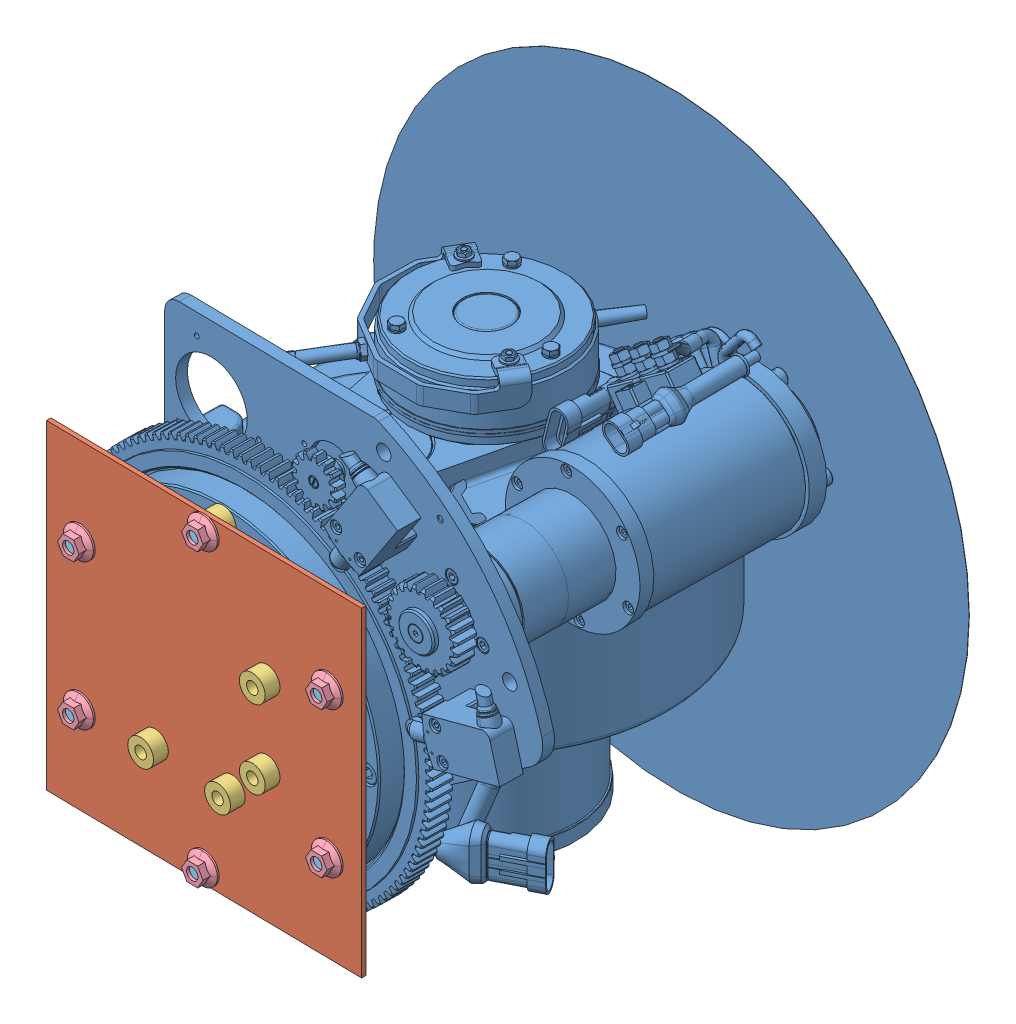
SolidWorks assembly motore+supporto, configuration Default. Lengths in mm.
Overall size (415.84 415.9 330.44).
29 component instances, 5 part files, 56 mates.
Components (placement in the parent):
- MR240FRS-AC.stp-1: MR240FRS-AC.stp [Default] at (480.9296 100.5307 -916.9118) size (415.84 415.9 312.91)
- supporto_motore-2: supporto_motore [Default] at (5.5916 0.2825 575.9688) x (-0.999869 0 -0.016207) z (0.016207 -0.000006 -0.999869) size (220 220 3)
- distanziale-1: distanziale [Default] at (92.3448 50.2824 567.3735) x (0.92025 -0.391047 0.014919) z (-0.016207 0.000006 0.999869) size (18 18 10)
- distanziale-2: distanziale [Default] at (-80.8375 -49.7176 564.5668) x (-0.654362 0.756107 -0.010611) z (-0.016207 0.000006 0.999869) size (18 18 10)
- distanziale-3: distanziale [Default] at (5.7536 -99.7176 565.9707) x (-0.654362 0.756107 -0.010611) z (-0.016207 0.000006 0.999869) size (18 18 10)
- distanziale-4: distanziale [Default] at (5.5916 100.2825 575.9683) x (-0.701568 -0.712512 -0.011368) z (0.016207 -0.000006 -0.999869) size (18 18 10)
- distanziale-5: distanziale [Default] at (92.3448 -49.7176 567.374) x (-0.654362 0.756107 -0.010611) z (-0.016207 0.000006 0.999869) size (18 18 10)
- distanziale-6: distanziale [Default] at (-80.8375 50.2824 564.5663) x (0.92025 -0.391047 0.014919) z (-0.016207 0.000006 0.999869) size (18 18 10)
- distanziale-7: distanziale [Default] at (-28.6146 -43.7175 588.4163) x (0.316566 0.948557 0.005126) z (0.016207 -0.000006 -0.999869) size (18 18 10)
- distanziale-8: distanziale [Default] at (49.3751 34.2825 589.6801) x (0.316566 0.948557 0.005126) z (0.016207 -0.000006 -0.999869) size (18 18 10)
- distanziale-9: distanziale [Default] at (25.1283 -43.7175 589.2875) x (-0.701568 -0.712512 -0.011368) z (0.016207 -0.000006 -0.999869) size (18 18 10)
- FLANGE_NUT_M8-1: FLANGE_NUT_M8 [Default] at (92.1341 -49.7175 580.3723) x (0.999869 0 0.016207) z (-0.016207 0.000006 0.999869) size (21 21 8)
- FLANGE_NUT_M8-2: FLANGE_NUT_M8 [Default] at (-81.0482 50.2825 577.5646) x (0.999869 0 0.016207) z (-0.016207 0.000006 0.999869) size (21 21 8)
- FLANGE_NUT_M8-3: FLANGE_NUT_M8 [Default] at (-81.0482 -49.7175 577.5651) x (0.999869 0 0.016207) z (-0.016207 0.000006 0.999869) size (21 21 8)
- FLANGE_NUT_M8-4: FLANGE_NUT_M8 [Default] at (5.5429 -99.7175 578.969) x (0.999869 0 0.016207) z (-0.016207 0.000006 0.999869) size (21 21 8)
- FLANGE_NUT_M8-5: FLANGE_NUT_M8 [Default] at (5.543 100.2825 578.9679) x (0.999869 0 0.016207) z (-0.016207 0.000006 0.999869) size (21 21 8)
- FLANGE_NUT_M8-6: FLANGE_NUT_M8 [Default] at (92.1342 50.2825 580.3717) x (0.999869 0 0.016207) z (-0.016207 0.000006 0.999869) size (21 21 8)
- FLANGE_NUT_M8-7: FLANGE_NUT_M8 [Default] at (-28.4039 -43.7175 575.418) x (-0.924292 -0.381392 -0.01498) z (0.016207 -0.000006 -0.999869) size (21 21 8)
- FLANGE_NUT_M8-8: FLANGE_NUT_M8 [Default] at (25.339 -43.7175 576.2892) x (0.999868 -0.000687 0.016207) z (0.016207 -0.000006 -0.999869) size (21 21 8)
- FLANGE_NUT_M8-9: FLANGE_NUT_M8 [Default] at (49.5858 34.2825 576.6818) x (-0.924292 -0.381392 -0.01498) z (0.016207 -0.000006 -0.999869) size (21 21 8)
- slotted countersunk flat head screw_iso-1: slotted countersunk flat head screw_iso [ISO 2009 - M8 x 50 - 38N] at (-80.3351 -49.7178 533.5709) x (-0.016207 0.000006 0.999869) z (-0.999869 -0.000006 -0.016207) size (50 15.8 15.67)
- slotted countersunk flat head screw_iso-2: slotted countersunk flat head screw_iso [ISO 2009 - M8 x 50 - 38N] at (-3.804 -13.9391 527.2162) size (50 15.8 15.67)
- slotted countersunk flat head screw_iso-4: slotted countersunk flat head screw_iso [ISO 2009 - M8 x 50 - 38N] at (6.2561 -99.7178 534.9748) x (-0.016207 0.000006 0.999869) z (-0.999869 -0.000006 -0.016207) size (50 15.8 15.67)
- slotted countersunk flat head screw_iso-5: slotted countersunk flat head screw_iso [ISO 2009 - M8 x 50 - 38N] at (92.8472 -49.7178 536.3781) x (-0.016207 0.000006 0.999869) z (-0.999869 -0.000006 -0.016207) size (50 15.8 15.67)
- slotted countersunk flat head screw_iso-6: slotted countersunk flat head screw_iso [ISO 2009 - M8 x 50 - 38N] at (-80.3351 50.2822 533.5704) x (-0.016207 0.000006 0.999869) z (-0.999869 -0.000006 -0.016207) size (50 15.8 15.67)
- slotted countersunk flat head screw_iso-7: slotted countersunk flat head screw_iso [ISO 2009 - M8 x 50 - 38N] at (6.2561 100.2822 534.9737) x (-0.016207 0.000006 0.999869) z (-0.999869 -0.000006 -0.016207) size (50 15.8 15.67)
- slotted countersunk flat head screw_iso-8: slotted countersunk flat head screw_iso [ISO 2009 - M8 x 50 - 38N] at (92.8473 50.2822 536.3775) x (-0.016207 0.000006 0.999869) z (-0.999869 -0.000006 -0.016207) size (50 15.8 15.67)
- distanziale-10: distanziale [Default] at (49.3751 -19.4675 589.6804) x (-0.807591 -0.589598 -0.013087) z (0.016207 -0.000006 -0.999869) size (18 18 10)
- FLANGE_NUT_M8-10: FLANGE_NUT_M8 [Default] at (49.5858 -19.4675 576.6821) x (-0.924292 -0.381392 -0.01498) z (0.016207 -0.000006 -0.999869) size (21 21 8)
Mates (geometry in assembly coordinates):
- Concentrico1: concentric aligned: cylinder of supporto_motore-2 through (92.1342 50.2825 580.3717) axis (0.016207 -0.000006 -0.999869) radius 4; cylinder of distanziale-1 through (92.1828 50.2824 577.3721) axis (0.016207 -0.000006 -0.999869) radius 4
- Coincidente1: coincident anti-aligned: plane of supporto_motore-2 through (5.5916 0.2825 575.9688) normal (0.016207 -0.000006 -0.999869); plane of distanziale-1 through (92.1828 50.2824 577.3721) normal (-0.016207 0.000006 0.999869)
- Coincidente2: coincident anti-aligned: plane of supporto_motore-2 through (5.5916 0.2825 575.9688) normal (0.016207 -0.000006 -0.999869); plane of distanziale-4 through (5.5916 100.2825 575.9683) normal (-0.016207 0.000006 0.999869)
- Concentrico2: concentric anti-aligned: cylinder of supporto_motore-2 through (5.543 100.2825 578.9679) axis (0.016207 -0.000006 -0.999869) radius 4; cylinder of distanziale-4 through (5.7537 100.2824 565.9696) axis (-0.016207 0.000006 0.999869) radius 4
- Coincidente3: coincident anti-aligned: plane of supporto_motore-2 through (5.5916 0.2825 575.9688) normal (0.016207 -0.000006 -0.999869); plane of distanziale-6 through (-80.9996 50.2825 574.565) normal (-0.016207 0.000006 0.999869)
- Concentrico3: concentric aligned: cylinder of supporto_motore-2 through (-81.0482 50.2825 577.5646) axis (0.016207 -0.000006 -0.999869) radius 4; cylinder of distanziale-6 through (-80.9996 50.2825 574.565) axis (0.016207 -0.000006 -0.999869) radius 4
- Concentrico4: concentric aligned: cylinder of supporto_motore-2 through (-81.0482 -49.7175 577.5651) axis (0.016207 -0.000006 -0.999869) radius 4; cylinder of distanziale-2 through (-80.9996 -49.7175 574.5655) axis (0.016207 -0.000006 -0.999869) radius 4
- Coincidente4: coincident anti-aligned: plane of supporto_motore-2 through (5.5916 0.2825 575.9688) normal (0.016207 -0.000006 -0.999869); plane of distanziale-2 through (-80.9996 -49.7175 574.5655) normal (-0.016207 0.000006 0.999869)
- Coincidente5: coincident anti-aligned: plane of supporto_motore-2 through (5.5916 0.2825 575.9688) normal (0.016207 -0.000006 -0.999869); plane of distanziale-3 through (5.5916 -99.7175 575.9694) normal (-0.016207 0.000006 0.999869)
- Concentrico5: concentric aligned: cylinder of supporto_motore-2 through (5.5429 -99.7175 578.969) axis (0.016207 -0.000006 -0.999869) radius 4; cylinder of distanziale-3 through (5.5916 -99.7175 575.9694) axis (0.016207 -0.000006 -0.999869) radius 4
- Coincidente6: coincident anti-aligned: plane of supporto_motore-2 through (5.5916 0.2825 575.9688) normal (0.016207 -0.000006 -0.999869); plane of distanziale-5 through (92.1827 -49.7176 577.3727) normal (-0.016207 0.000006 0.999869)
- Concentrico6: concentric aligned: cylinder of supporto_motore-2 through (92.1341 -49.7175 580.3723) axis (0.016207 -0.000006 -0.999869) radius 4; cylinder of distanziale-5 through (92.1827 -49.7176 577.3727) axis (0.016207 -0.000006 -0.999869) radius 4
- Concentrico7: concentric anti-aligned: cylinder of MR240FRS-AC.stp-1 through (10.7642 -99.7193 256.856) axis (-0.016207 0.000006 0.999869) radius 3.3235; cylinder of distanziale-3 through (5.5916 -99.7175 575.9694) axis (0.016207 -0.000006 -0.999869) radius 4
- Concentrico8: concentric aligned: cylinder of MR240FRS-AC.stp-1 through (10.7642 100.2807 256.8549) axis (-0.016207 0.000006 0.999869) radius 3.3235; cylinder of distanziale-4 through (5.7537 100.2824 565.9696) axis (-0.016207 0.000006 0.999869) radius 4
- Coincidente7: coincident anti-aligned: plane of MR240FRS-AC.stp-1 through (102.7409 0.2824 567.5422) normal (-0.016207 0.000006 0.999869); plane of distanziale-3 through (5.7536 -99.7176 565.9707) normal (0.016207 -0.000006 -0.999869)
- Coincidente9: coincident anti-aligned: plane of supporto_motore-2 through (5.543 0.2825 578.9684) normal (-0.016207 0.000006 0.999869); plane of distanziale-8 through (49.5372 34.2825 579.6814) normal (0.016207 -0.000006 -0.999869)
- Coincidente10: coincident anti-aligned: plane of supporto_motore-2 through (5.543 0.2825 578.9684) normal (-0.016207 0.000006 0.999869); plane of distanziale-7 through (-28.4526 -43.7175 578.4176) normal (0.016207 -0.000006 -0.999869)
- Coincidente11: coincident anti-aligned: plane of supporto_motore-2 through (5.543 0.2825 578.9684) normal (-0.016207 0.000006 0.999869); plane of distanziale-9 through (25.2904 -43.7175 579.2888) normal (0.016207 -0.000006 -0.999869)
- Concentrico10: concentric anti-aligned: cylinder of supporto_motore-2 through (-28.4526 -43.7175 578.4176) axis (0.016207 -0.000006 -0.999869) radius 4; cylinder of distanziale-7 through (-28.4526 -43.7175 578.4176) axis (-0.016207 0.000006 0.999869) radius 4
- Concentrico11: concentric anti-aligned: cylinder of supporto_motore-2 through (25.2904 -43.7175 579.2888) axis (0.016207 -0.000006 -0.999869) radius 4; cylinder of distanziale-9 through (25.2904 -43.7175 579.2888) axis (-0.016207 0.000006 0.999869) radius 4
- Concentrico12: concentric anti-aligned: cylinder of supporto_motore-2 through (49.5372 34.2825 579.6814) axis (0.016207 -0.000006 -0.999869) radius 4; cylinder of distanziale-8 through (49.5372 34.2825 579.6814) axis (-0.016207 0.000006 0.999869) radius 4
- Concentrico13: concentric aligned: cylinder of supporto_motore-2 through (25.2904 -43.7175 579.2888) axis (0.016207 -0.000006 -0.999869) radius 4; cylinder of FLANGE_NUT_M8-8 through (25.4751 -43.7176 567.8903) axis (0.016207 -0.000006 -0.999869) radius 4
- Coincidente12: coincident anti-aligned: plane of supporto_motore-2 through (5.5916 0.2825 575.9688) normal (0.016207 -0.000006 -0.999869); plane of FLANGE_NUT_M8-8 through (36.8954 -32.1755 576.4764) normal (-0.016207 0.000006 0.999869)
- Coincidente13: coincident anti-aligned: plane of supporto_motore-2 through (5.5916 0.2825 575.9688) normal (0.016207 -0.000006 -0.999869); plane of FLANGE_NUT_M8-9 through (43.3148 19.2004 576.5802) normal (-0.016207 0.000006 0.999869)
- Concentrico14: concentric aligned: cylinder of supporto_motore-2 through (49.5372 34.2825 579.6814) axis (0.016207 -0.000006 -0.999869) radius 4; cylinder of FLANGE_NUT_M8-9 through (49.722 34.2824 568.2829) axis (0.016207 -0.000006 -0.999869) radius 4
- Coincidente14: coincident anti-aligned: plane of supporto_motore-2 through (5.5916 0.2825 575.9688) normal (0.016207 -0.000006 -0.999869); plane of FLANGE_NUT_M8-7 through (-34.675 -58.7996 575.3165) normal (-0.016207 0.000006 0.999869)
- Concentrico15: concentric aligned: cylinder of supporto_motore-2 through (-28.4526 -43.7175 578.4176) axis (0.016207 -0.000006 -0.999869) radius 4; cylinder of FLANGE_NUT_M8-7 through (-28.2678 -43.7176 567.0191) axis (0.016207 -0.000006 -0.999869) radius 4
- Coincidente15: coincident anti-aligned: plane of supporto_motore-2 through (5.543 0.2825 578.9684) normal (-0.016207 0.000006 0.999869); plane of FLANGE_NUT_M8-4 through (17.0914 -111.2675 579.1563) normal (0.016207 -0.000006 -0.999869)
- Coincidente16: coincident anti-aligned: plane of supporto_motore-2 through (5.543 0.2825 578.9684) normal (-0.016207 0.000006 0.999869); plane of FLANGE_NUT_M8-1 through (103.6826 -61.2675 580.5596) normal (0.016207 -0.000006 -0.999869)
- Coincidente17: coincident anti-aligned: plane of supporto_motore-2 through (5.543 0.2825 578.9684) normal (-0.016207 0.000006 0.999869); plane of FLANGE_NUT_M8-5 through (17.0915 88.7325 579.1551) normal (0.016207 -0.000006 -0.999869)
- Coincidente18: coincident anti-aligned: plane of supporto_motore-2 through (5.543 0.2825 578.9684) normal (-0.016207 0.000006 0.999869); plane of FLANGE_NUT_M8-6 through (103.6826 38.7325 580.559) normal (0.016207 -0.000006 -0.999869)
- Coincidente19: coincident anti-aligned: plane of supporto_motore-2 through (5.543 0.2825 578.9684) normal (-0.016207 0.000006 0.999869); plane of FLANGE_NUT_M8-3 through (-69.4997 -61.2675 577.7524) normal (0.016207 -0.000006 -0.999869)
- Coincidente20: coincident anti-aligned: plane of supporto_motore-2 through (5.543 0.2825 578.9684) normal (-0.016207 0.000006 0.999869); plane of FLANGE_NUT_M8-2 through (-69.4997 38.7325 577.7518) normal (0.016207 -0.000006 -0.999869)
- Concentrico16: concentric anti-aligned: cylinder of supporto_motore-2 through (-81.0482 -49.7175 577.5651) axis (0.016207 -0.000006 -0.999869) radius 4; cylinder of FLANGE_NUT_M8-3 through (-81.1843 -49.7175 585.964) axis (-0.016207 0.000006 0.999869) radius 4
- Concentrico17: concentric anti-aligned: cylinder of supporto_motore-2 through (-81.0482 50.2825 577.5646) axis (0.016207 -0.000006 -0.999869) radius 4; cylinder of FLANGE_NUT_M8-2 through (-81.1843 50.2825 585.9635) axis (-0.016207 0.000006 0.999869) radius 4
- Concentrico18: concentric anti-aligned: cylinder of supporto_motore-2 through (5.543 100.2825 578.9679) axis (0.016207 -0.000006 -0.999869) radius 4; cylinder of FLANGE_NUT_M8-5 through (5.4069 100.2825 587.3668) axis (-0.016207 0.000006 0.999869) radius 4
- Concentrico19: concentric anti-aligned: cylinder of supporto_motore-2 through (92.1342 50.2825 580.3717) axis (0.016207 -0.000006 -0.999869) radius 4; cylinder of FLANGE_NUT_M8-6 through (91.998 50.2825 588.7706) axis (-0.016207 0.000006 0.999869) radius 4
- Concentrico20: concentric anti-aligned: cylinder of supporto_motore-2 through (92.1341 -49.7175 580.3723) axis (0.016207 -0.000006 -0.999869) radius 4; cylinder of FLANGE_NUT_M8-1 through (91.998 -49.7175 588.7712) axis (-0.016207 0.000006 0.999869) radius 4
- Concentrico21: concentric anti-aligned: cylinder of supporto_motore-2 through (5.5429 -99.7175 578.969) axis (0.016207 -0.000006 -0.999869) radius 4; cylinder of FLANGE_NUT_M8-4 through (5.4068 -99.7175 587.3679) axis (-0.016207 0.000006 0.999869) radius 4
- Concentrico22: concentric aligned: cylinder of MR240FRS-AC.stp-1 through (-74.6264 -49.7197 181.3862) axis (-0.016207 0.000006 0.999869) radius 4.5; cone of slotted countersunk flat head screw_iso-1 through (-80.3472 -49.7177 534.3208) axis (-0.016207 0.000006 0.999869)
- Coincidente21: coincident aligned: plane of MR240FRS-AC.stp-1 through (-94.2307 0.2823 533.3454) normal (0.016207 -0.000006 -0.999869); plane of slotted countersunk flat head screw_iso-1 through (-80.3351 -49.7178 533.5709) normal (0.016207 -0.000006 -0.999869)
- Concentrico23: concentric aligned: cylinder of MR240FRS-AC.stp-1 through (11.9647 -99.7197 182.7901) axis (-0.016207 0.000006 0.999869) radius 4.5; cone of slotted countersunk flat head screw_iso-4 through (6.2439 -99.7178 535.7247) axis (-0.016207 0.000006 0.999869)
- Concentrico24: concentric aligned: cylinder of MR240FRS-AC.stp-1 through (98.5559 -49.7197 184.1934) axis (-0.016207 0.000006 0.999869) radius 4.5; cone of slotted countersunk flat head screw_iso-5 through (92.8351 -49.7178 537.128) axis (-0.016207 0.000006 0.999869)
- Concentrico25: concentric aligned: cylinder of MR240FRS-AC.stp-1 through (-74.6264 50.2803 181.3857) axis (-0.016207 0.000006 0.999869) radius 4.5; cone of slotted countersunk flat head screw_iso-6 through (-80.3472 50.2823 534.3203) axis (-0.016207 0.000006 0.999869)
- Concentrico26: concentric aligned: cylinder of FLANGE_NUT_M8-5 through (5.4069 100.2825 587.3668) axis (-0.016207 0.000006 0.999869) radius 4; cone of slotted countersunk flat head screw_iso-7 through (6.244 100.2822 535.7236) axis (-0.016207 0.000006 0.999869)
- Concentrico27: concentric aligned: cylinder of FLANGE_NUT_M8-6 through (91.998 50.2825 588.7706) axis (-0.016207 0.000006 0.999869) radius 4; cone of slotted countersunk flat head screw_iso-8 through (92.8351 50.2822 537.1274) axis (-0.016207 0.000006 0.999869)
- Coincidente22: coincident aligned: plane of MR240FRS-AC.stp-1 through (-94.2307 0.2823 533.3454) normal (0.016207 -0.000006 -0.999869); plane of slotted countersunk flat head screw_iso-4 through (6.2561 -99.7178 534.9748) normal (0.016207 -0.000006 -0.999869)
- Coincidente23: coincident aligned: plane of MR240FRS-AC.stp-1 through (-94.2307 0.2823 533.3454) normal (0.016207 -0.000006 -0.999869); plane of slotted countersunk flat head screw_iso-6 through (-80.3351 50.2822 533.5704) normal (0.016207 -0.000006 -0.999869)
- Coincidente24: coincident aligned: plane of slotted countersunk flat head screw_iso-4 through (5.4457 -95.7175 584.9682) normal (-0.016207 0.000006 0.999869); plane of slotted countersunk flat head screw_iso-8 through (92.0369 54.2825 586.3709) normal (-0.016207 0.000006 0.999869)
- Coincidente25: coincident aligned: plane of slotted countersunk flat head screw_iso-4 through (5.4457 -95.7175 584.9682) normal (-0.016207 0.000006 0.999869); plane of slotted countersunk flat head screw_iso-7 through (5.4457 104.2825 584.9671) normal (-0.016207 0.000006 0.999869)
- Coincidente26: coincident aligned: plane of slotted countersunk flat head screw_iso-4 through (5.4457 -95.7175 584.9682) normal (-0.016207 0.000006 0.999869); plane of slotted countersunk flat head screw_iso-6 through (-81.1454 54.2825 583.5638) normal (-0.016207 0.000006 0.999869)
- Coincidente27: coincident aligned: plane of MR240FRS-AC.stp-1 through (-94.2307 0.2823 533.3454) normal (0.016207 -0.000006 -0.999869); plane of slotted countersunk flat head screw_iso-5 through (92.8472 -49.7178 536.3781) normal (0.016207 -0.000006 -0.999869)
- Concentrico28: concentric anti-aligned: cylinder of supporto_motore-2 through (49.5372 -19.4675 579.6817) axis (0.016207 -0.000006 -0.999869) radius 4; cylinder of distanziale-10 through (49.5372 -19.4675 579.6817) axis (-0.016207 0.000006 0.999869) radius 4
- Coincidente28: coincident anti-aligned: plane of supporto_motore-2 through (5.543 0.2825 578.9684) normal (-0.016207 0.000006 0.999869); plane of distanziale-10 through (49.5372 -19.4675 579.6817) normal (0.016207 -0.000006 -0.999869)
- Concentrico29: concentric aligned: cylinder of supporto_motore-2 through (49.5372 -19.4675 579.6817) axis (0.016207 -0.000006 -0.999869) radius 4; cylinder of FLANGE_NUT_M8-10 through (49.722 -19.4676 568.2832) axis (0.016207 -0.000006 -0.999869) radius 4
- Coincidente29: coincident anti-aligned: plane of supporto_motore-2 through (5.5916 0.2825 575.9688) normal (0.016207 -0.000006 -0.999869); plane of FLANGE_NUT_M8-10 through (43.3147 -34.5496 576.5805) normal (-0.016207 0.000006 0.999869)
